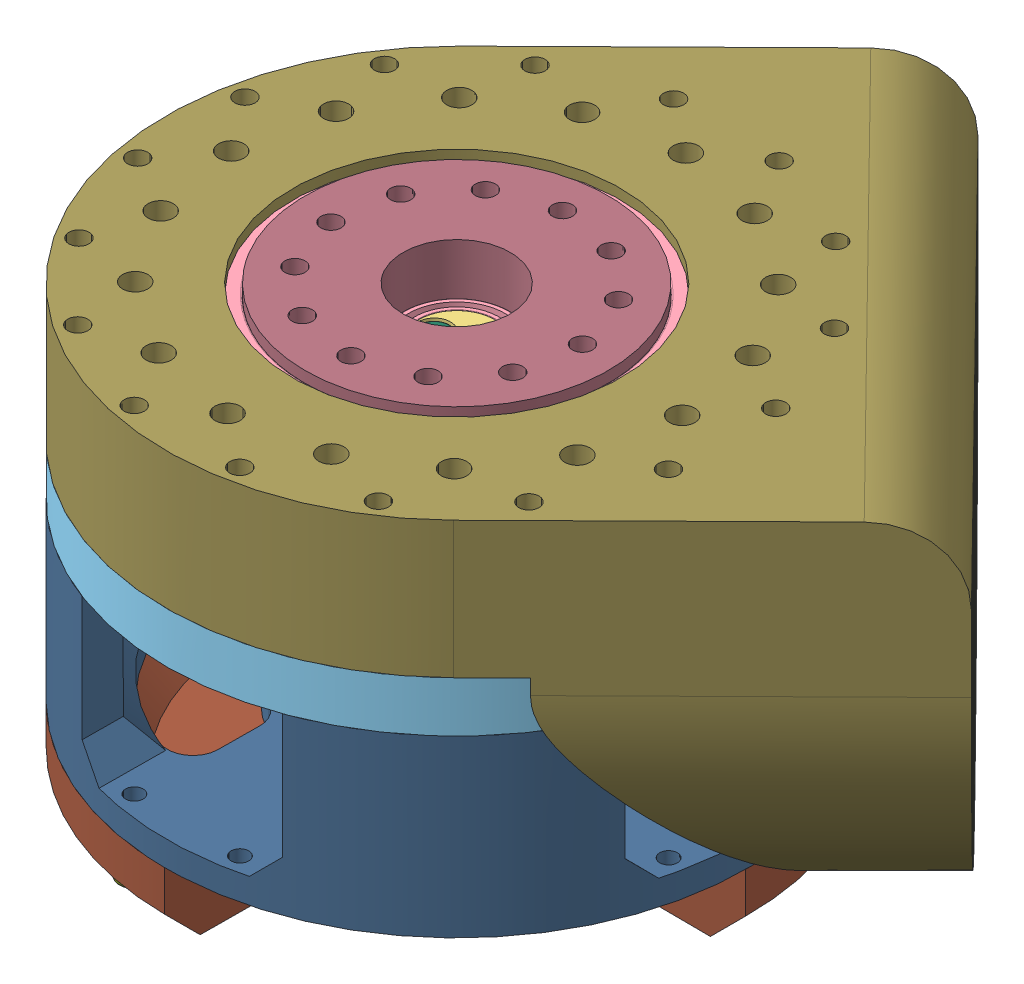
SolidWorks assembly Cycloidal _v3, configuration Default. Lengths in mm.
Overall size (173.36 87.57 173.15).
95 component instances, 17 part files, 90 mates.
Components (placement in the parent):
- motor-X83008S.stp-1: motor-X83008S.stp [Default] at (3.9105 88.7742 94.1058) x (0.928336 0.00037 -0.371741) z (0.000399 -1 0) (suppressed, hidden)
- Base_Plate-1: Base_Plate [Default] at (47.4533 68.6574 89.6282) x (-0.992404 -0.000396 0.123023) z (-0.123023 -0.000049 -0.992404) size (39.8 11 39.8)
- Eccentric_Shaft-1: Eccentric_Shaft [Default] at (60.4961 73.3217 80.3225) x (0.123023 0.000049 0.992404) z (-0.992404 -0.000396 0.123023) size (20 17 17)
  - Eccentric_Shaft_bot-1: Eccentric_Shaft_bot [Default] at (7.6302 12.3409 14.0904) x (1 0 0) z (0 0 -1) size (17 6 17)
  - Eccentric_Shaft_bot-2: Eccentric_Shaft_bot [Default] at (7.6302 12.3409 14.0904) x (-1 0 0) z (0 0 -1) size (17 6 17)
  - Eccentric_Shaft_top-1: Eccentric_Shaft_top [Default] at (7.6302 18.3409 14.0904) x (-1 0 0) z (0 0 -1) size (17 5 17)
- radial ball bearing_68_iso-39: radial ball bearing_68_iso [ISO 15 RBB - 1860 - 32,SI,NC,32_68] at (47.4409 99.6574 89.6282) x (0.000399 -1 0) z (-0.546908 -0.000218 0.837193) size (10 78 78)
- radial ball bearing_68_iso-40: radial ball bearing_68_iso [ISO 15 RBB - 1840 - 32,SI,NC,32_68] at (47.4516 72.9574 89.6282) x (-0.000399 1 0) z (0.001003 0 0.999999) size (7 52 52)
- Base_plate_2-1: Base_plate_2 [Default] at (47.4529 69.6574 89.6282) x (0.712755 0.000284 -0.701413) z (0.701413 0.00028 0.712755) size (115 10 115)
- m13_bearing-31: m13_bearing [Default] at (-10.4263 95.4017 67.196) x (0.227678 0.000091 0.973736) z (0.973736 0.000388 -0.227678) size (13 16 13)
  - m6-1: m6 [Default] at (8.4921 2.5508 14.8914) size (6 16 6)
  - radial ball bearing_68_iso-1: radial ball bearing_68_iso [ISO 15 RBB - 286 - 10,SI,NC,10_68] at (8.4921 16.0508 14.8914) x (0 1 0) z (0 0 1) size (5 13 13)
  - radial ball bearing_68_iso-2: radial ball bearing_68_iso [ISO 15 RBB - 286 - 10,SI,NC,10_68] at (8.4921 11.0508 14.8914) x (0 1 0) z (0 0 1) size (5 13 13)
- m13_bearing-32: m13_bearing [Default] at (-13.9908 98.1837 84.3887) x (0.227678 0.000091 0.973736) z (0.973736 0.000388 -0.227678) size (13 16 13)
  - m6-1: m6 [Default] at (8.4921 2.5508 14.8914) size (6 16 6)
  - radial ball bearing_68_iso-1: radial ball bearing_68_iso [ISO 15 RBB - 286 - 10,SI,NC,10_68] at (8.4921 16.0508 14.8914) x (0 1 0) z (0 0 1) size (5 13 13)
  - radial ball bearing_68_iso-2: radial ball bearing_68_iso [ISO 15 RBB - 286 - 10,SI,NC,10_68] at (8.4921 11.0508 14.8914) x (0 1 0) z (0 0 1) size (5 13 13)
- m13_bearing-34: m13_bearing [Default] at (13.4541 98.1947 126.1847) x (0.227678 0.000091 0.973736) z (0.973736 0.000388 -0.227678) size (13 16 13)
  - m6-1: m6 [Default] at (8.4921 2.5508 14.8914) size (6 16 6)
  - radial ball bearing_68_iso-1: radial ball bearing_68_iso [ISO 15 RBB - 286 - 10,SI,NC,10_68] at (8.4921 16.0508 14.8914) x (0 1 0) z (0 0 1) size (5 13 13)
  - radial ball bearing_68_iso-2: radial ball bearing_68_iso [ISO 15 RBB - 286 - 10,SI,NC,10_68] at (8.4921 11.0508 14.8914) x (0 1 0) z (0 0 1) size (5 13 13)
- m13_bearing-35: m13_bearing [Default] at (-1.0662 98.1889 116.3132) x (0.227678 0.000091 0.973736) z (0.973736 0.000388 -0.227678) size (13 16 13)
  - m6-1: m6 [Default] at (8.4921 2.5508 14.8914) size (6 16 6)
  - radial ball bearing_68_iso-1: radial ball bearing_68_iso [ISO 15 RBB - 286 - 10,SI,NC,10_68] at (8.4921 16.0508 14.8914) x (0 1 0) z (0 0 1) size (5 13 13)
  - radial ball bearing_68_iso-2: radial ball bearing_68_iso [ISO 15 RBB - 286 - 10,SI,NC,10_68] at (8.4921 11.0508 14.8914) x (0 1 0) z (0 0 1) size (5 13 13)
- m13_bearing-36: m13_bearing [Default] at (-10.7036 98.185 101.6364) x (0.227678 0.000091 0.973736) z (0.973736 0.000388 -0.227678) size (13 16 13)
  - m6-1: m6 [Default] at (8.4921 2.5508 14.8914) size (6 16 6)
  - radial ball bearing_68_iso-1: radial ball bearing_68_iso [ISO 15 RBB - 286 - 10,SI,NC,10_68] at (8.4921 16.0508 14.8914) x (0 1 0) z (0 0 1) size (5 13 13)
  - radial ball bearing_68_iso-2: radial ball bearing_68_iso [ISO 15 RBB - 286 - 10,SI,NC,10_68] at (8.4921 11.0508 14.8914) x (0 1 0) z (0 0 1) size (5 13 13)
- m13_bearing-1: m13_bearing [Default] at (-0.4494 98.1891 62.778) x (0.736525 0.000294 0.676411) z (0.676411 0.00027 -0.736525) size (13 16 13)
  - m6-1: m6 [Default] at (8.4921 2.5508 14.8914) size (6 16 6)
  - radial ball bearing_68_iso-1: radial ball bearing_68_iso [ISO 15 RBB - 286 - 10,SI,NC,10_68] at (8.4921 16.0508 14.8914) x (0 1 0) z (0 0 1) size (5 13 13)
  - radial ball bearing_68_iso-2: radial ball bearing_68_iso [ISO 15 RBB - 286 - 10,SI,NC,10_68] at (8.4921 11.0508 14.8914) x (0 1 0) z (0 0 1) size (5 13 13)
- m13_bearing-2: m13_bearing [Default] at (48.5236 98.2087 124.7001) x (0.120271 0.000048 0.992741) z (0.992741 0.000396 -0.120271) size (13 16 13)
  - m6-1: m6 [Default] at (8.4921 2.5508 14.8914) size (6 16 6)
  - radial ball bearing_68_iso-1: radial ball bearing_68_iso [ISO 15 RBB - 286 - 10,SI,NC,10_68] at (8.4921 16.0508 14.8914) x (0 1 0) z (0 0 1) size (5 13 13)
  - radial ball bearing_68_iso-2: radial ball bearing_68_iso [ISO 15 RBB - 286 - 10,SI,NC,10_68] at (8.4921 11.0508 14.8914) x (0 1 0) z (0 0 1) size (5 13 13)
- m13_bearing-3: m13_bearing [Default] at (32.5019 98.2023 52.3604) x (0.833889 0.000333 0.551933) z (0.551932 0.00022 -0.833889) size (13 16 13)
  - m6-1: m6 [Default] at (8.4921 2.5508 14.8914) size (6 16 6)
  - radial ball bearing_68_iso-1: radial ball bearing_68_iso [ISO 15 RBB - 286 - 10,SI,NC,10_68] at (8.4921 16.0508 14.8914) x (0 1 0) z (0 0 1) size (5 13 13)
  - radial ball bearing_68_iso-2: radial ball bearing_68_iso [ISO 15 RBB - 286 - 10,SI,NC,10_68] at (8.4921 11.0508 14.8914) x (0 1 0) z (0 0 1) size (5 13 13)
- m13_bearing-4: m13_bearing [Default] at (77.3632 98.2202 81.8307) x (0.022268 0.000009 0.999752) z (0.999752 0.000399 -0.022268) size (13 16 13)
  - m6-1: m6 [Default] at (8.4921 2.5508 14.8914) size (6 16 6)
  - radial ball bearing_68_iso-1: radial ball bearing_68_iso [ISO 15 RBB - 286 - 10,SI,NC,10_68] at (8.4921 16.0508 14.8914) x (0 1 0) z (0 0 1) size (5 13 13)
  - radial ball bearing_68_iso-2: radial ball bearing_68_iso [ISO 15 RBB - 286 - 10,SI,NC,10_68] at (8.4921 11.0508 14.8914) x (0 1 0) z (0 0 1) size (5 13 13)
- m13_bearing-5: m13_bearing [Default] at (73.5091 98.2186 99.5852) x (0.059133 0.000024 0.99825) z (0.99825 0.000398 -0.059133) size (13 16 13)
  - m6-1: m6 [Default] at (8.4921 2.5508 14.8914) size (6 16 6)
  - radial ball bearing_68_iso-1: radial ball bearing_68_iso [ISO 15 RBB - 286 - 10,SI,NC,10_68] at (8.4921 16.0508 14.8914) x (0 1 0) z (0 0 1) size (5 13 13)
  - radial ball bearing_68_iso-2: radial ball bearing_68_iso [ISO 15 RBB - 286 - 10,SI,NC,10_68] at (8.4921 11.0508 14.8914) x (0 1 0) z (0 0 1) size (5 13 13)
- m13_bearing-6: m13_bearing [Default] at (13.4333 98.1947 47.0643) x (0.451561 0.00018 0.89224) z (0.89224 0.000356 -0.451561) size (13 16 13)
  - m6-1: m6 [Default] at (8.4921 2.5508 14.8914) size (6 16 6)
  - radial ball bearing_68_iso-1: radial ball bearing_68_iso [ISO 15 RBB - 286 - 10,SI,NC,10_68] at (8.4921 16.0508 14.8914) x (0 1 0) z (0 0 1) size (5 13 13)
  - radial ball bearing_68_iso-2: radial ball bearing_68_iso [ISO 15 RBB - 286 - 10,SI,NC,10_68] at (8.4921 11.0508 14.8914) x (0 1 0) z (0 0 1) size (5 13 13)
- m13_bearing-7: m13_bearing [Default] at (57.1526 98.2121 32.9496) x (-0.545813 -0.000218 0.837907) z (0.837907 0.000334 0.545813) size (13 16 13)
  - m6-1: m6 [Default] at (8.4921 2.5508 14.8914) size (6 16 6)
  - radial ball bearing_68_iso-1: radial ball bearing_68_iso [ISO 15 RBB - 286 - 10,SI,NC,10_68] at (8.4921 16.0508 14.8914) x (0 1 0) z (0 0 1) size (5 13 13)
  - radial ball bearing_68_iso-2: radial ball bearing_68_iso [ISO 15 RBB - 286 - 10,SI,NC,10_68] at (8.4921 11.0508 14.8914) x (0 1 0) z (0 0 1) size (5 13 13)
- m13_bearing-8: m13_bearing [Default] at (73.1034 98.2185 66.7178) x (0.158553 0.000063 0.98735) z (0.98735 0.000394 -0.158553) size (13 16 13)
  - m6-1: m6 [Default] at (8.4921 2.5508 14.8914) size (6 16 6)
  - radial ball bearing_68_iso-1: radial ball bearing_68_iso [ISO 15 RBB - 286 - 10,SI,NC,10_68] at (8.4921 16.0508 14.8914) x (0 1 0) z (0 0 1) size (5 13 13)
  - radial ball bearing_68_iso-2: radial ball bearing_68_iso [ISO 15 RBB - 286 - 10,SI,NC,10_68] at (8.4921 11.0508 14.8914) x (0 1 0) z (0 0 1) size (5 13 13)
- m13_bearing-9: m13_bearing [Default] at (74.5316 98.219 41.6624) x (-0.687134 -0.000274 0.72653) z (0.72653 0.00029 0.687134) size (13 16 13)
  - m6-1: m6 [Default] at (8.4921 2.5508 14.8914) size (6 16 6)
  - radial ball bearing_68_iso-1: radial ball bearing_68_iso [ISO 15 RBB - 286 - 10,SI,NC,10_68] at (8.4921 16.0508 14.8914) x (0 1 0) z (0 0 1) size (5 13 13)
  - radial ball bearing_68_iso-2: radial ball bearing_68_iso [ISO 15 RBB - 286 - 10,SI,NC,10_68] at (8.4921 11.0508 14.8914) x (0 1 0) z (0 0 1) size (5 13 13)
- m13_bearing-11: m13_bearing [Default] at (30.0113 98.2013 136.2104) x (0.57351 0.000229 0.819198) z (0.819198 0.000327 -0.57351) size (13 16 13)
  - m6-1: m6 [Default] at (8.4921 2.5508 14.8914) size (6 16 6)
  - radial ball bearing_68_iso-1: radial ball bearing_68_iso [ISO 15 RBB - 286 - 10,SI,NC,10_68] at (8.4921 16.0508 14.8914) x (0 1 0) z (0 0 1) size (5 13 13)
  - radial ball bearing_68_iso-2: radial ball bearing_68_iso [ISO 15 RBB - 286 - 10,SI,NC,10_68] at (8.4921 11.0508 14.8914) x (0 1 0) z (0 0 1) size (5 13 13)
- m13_bearing-12: m13_bearing [Default] at (62.5932 98.2143 116.7506) x (0.22335 0.000089 0.974738) z (0.974738 0.000389 -0.22335) size (13 16 13)
  - m6-1: m6 [Default] at (8.4921 2.5508 14.8914) size (6 16 6)
  - radial ball bearing_68_iso-1: radial ball bearing_68_iso [ISO 15 RBB - 286 - 10,SI,NC,10_68] at (8.4921 16.0508 14.8914) x (0 1 0) z (0 0 1) size (5 13 13)
  - radial ball bearing_68_iso-2: radial ball bearing_68_iso [ISO 15 RBB - 286 - 10,SI,NC,10_68] at (8.4921 11.0508 14.8914) x (0 1 0) z (0 0 1) size (5 13 13)
- M3x4x4.2_brass_insert-22: M3x4x4.2_brass_insert [Default] at (43.4837 68.6558 90.1203) x (0.984609 0.000393 -0.174769) z (0.174769 0.00007 0.984609) size (4 4 4)
- M3x4x4.2_brass_insert-23: M3x4x4.2_brass_insert [Default] at (51.4229 68.659 89.1361) x (0.984609 0.000393 -0.174769) z (0.174769 0.00007 0.984609) size (4 4 4)
- radial ball bearing_68_iso-44: radial ball bearing_68_iso [ISO 15 RBB - 1715 - 26,SI,NC,26_68] at (47.2636 81.6573 88.1396) x (0.000399 -1 0) z (0.171535 0.000068 0.985178) size (4 21 21)
- radial ball bearing_68_iso-45: radial ball bearing_68_iso [ISO 15 RBB - 1715 - 26,SI,NC,26_68] at (47.4429 94.6574 89.6282) x (0.000399 -1 0) z (0.819169 0.000327 0.573552) size (4 21 21)
- radial ball bearing_68_iso-46: radial ball bearing_68_iso [ISO 15 RBB - 1715 - 26,SI,NC,26_68] at (47.6295 89.6575 91.1168) x (-0.000399 1 0) z (0 0 1) size (4 21 21)
- foc-motor-controller.step-1: foc-motor-controller.step [Default] at (47.4677 32.6574 89.6282) x (0.701413 0.00028 0.712755) z (0.000399 -1 0) (suppressed, hidden)
- hex nut style 1 gradeab_iso-1: hex nut style 1 gradeab_iso [ISO - 4032 - M3 - W - N] at (47.7115 32.6575 59.2236) x (1 0.000399 0) z (0.000399 -1 0) size (5.5 6.35 2.4)
- Cycloidal_Discs_8308-1: Cycloidal_Discs_8308 [Default] at (-11.9184 124.164 51.5043) x (0.028527 0.000011 0.999593) z (0.999593 0.000399 -0.028527) size (79.25 5 79.73)
  - Cycloidal_Discs-1: Cycloidal_Discs [Default] at (38.3081 39.5303 58.0959) size (79.25 5 79.73)
- Cycloidal_Discs_8308-2: Cycloidal_Discs_8308 [Default] at (62.1667 47.133 159.1742) x (-0.931329 -0.000371 -0.364178) z (0.364178 0.000145 -0.931329) size (79.25 5 79.73)
  - Cycloidal_Discs-1: Cycloidal_Discs [Default] at (38.3081 39.5303 58.0959) size (79.25 5 79.73)
- Motor_Cover_v2-2: Motor_Cover_v2 [Default] at (47.4667 35.0574 89.6282) x (0.999968 0.000399 0.00802) z (-0.00802 -0.000003 0.999968) size (115 34.6 115)
- driver_cover-1: driver_cover [Default] at (47.4667 35.0574 89.6282) x (0.702656 0.00028 0.711529) z (0.711529 0.000284 -0.702656) size (81.32 15 115)
- Cover_new-1: Cover_new [Default] at (47.4437 92.6574 89.6282) x (0.701413 0.00028 0.712755) z (-0.712755 -0.000284 0.701413) size (115 87.5 130)
- Output_Shaft-2: Output_Shaft [Default] at (47.4437 92.6574 89.6282) x (0.572675 0.000228 0.819783) z (-0.819783 -0.000327 0.572675) size (70 14 70)
- radial ball bearing_68_iso-47: radial ball bearing_68_iso [ISO 15 RBB - 289 - 14,SI,NC,14_68] at (61.9924 89.1632 109.081) x (0.000399 -1 0) z (-0.055662 -0.000022 0.99845) size (5 17 17)
- radial ball bearing_68_iso-48: radial ball bearing_68_iso [ISO 15 RBB - 289 - 14,SI,NC,14_68] at (59.3269 82.1622 107.722) x (0.000399 -1 0) z (-0.055662 -0.000022 0.99845) size (5 17 17)
- m4x14-1: m4x14 [Default] at (47.0925 68.4573 134.6267) x (0.999623 0.000399 0.027466) z (-0.027466 -0.000011 0.999623) size (8 15.2 8)
- M3x20-1: M3x20 [Default] at (43.4726 96.3558 90.1203) x (-0.837193 -0.000334 -0.546908) z (-0.546908 -0.000218 0.837193) size (6 21.2 6)
- M3x10-1: M3x10 [Default] at (36.5111 25.853 142.5044) x (0.424034 0.000169 -0.905646) z (0.905646 0.000361 0.424034) size (6 11.2 6)
- m3x60-1: m3x60 [Default] at (17.1068 35.0453 134.2855) x (-0.837193 -0.000334 -0.546908) z (-0.546908 -0.000218 0.837193) size (5.3 63 5.3)
- m6-1: m6 [Default] at (60.6129 98.6627 108.4832) x (-0.153131 -0.000061 0.988206) z (0.988206 0.000394 0.153131) size (6 16 6)
Mates (geometry in assembly coordinates):
- Coincident1: coincident anti-aligned: plane of motor-X83008S.stp-1/outrunner.stp-1 through (51.6976 68.6591 123.8661) normal (-0.000399 1 0); plane of Base_Plate-1 through (47.4533 68.6574 89.6282) normal (0.000399 -1 0)
- Concentric1: concentric anti-aligned: line of motor-X83008S.stp-1/outrunner.stp-1 through (49.3624 63.1582 105.0104) axis (-0.000399 1 0); cylinder of Base_Plate-1 through (49.3558 79.6582 105.0104) axis (0.000399 -1 0) radius 2
- Concentric2: concentric anti-aligned: cylinder of motor-X83008S.stp-1/shaft.stp-1 through (47.4533 68.6574 89.6282) axis (-0.000399 1 0) radius 1.5; line of Base_Plate-1 through (47.4489 79.6574 89.6282) axis (0.000399 -1 0)
- Concentric78: concentric anti-aligned: cylinder of Base_Plate-1 through (47.4489 79.6574 89.6282) axis (0.000399 -1 0) radius 19.9; cylinder of radial ball bearing_68_iso-40 through (47.4598 52.3199 89.6282) axis (-0.000399 1 0) radius 20
- Concentric1437: concentric anti-aligned: cylinder of Base_Plate-1 through (43.4793 79.6558 90.1203) axis (0.000399 -1 0) radius 2; cylinder of M3x4x4.2_brass_insert-22 through (43.4817 73.5579 90.1203) axis (-0.000399 1 0) radius 1.5
- Coincident1479: coincident aligned: plane of Base_Plate-1 through (47.4533 68.6574 89.6282) normal (0.000399 -1 0); plane of M3x4x4.2_brass_insert-22 through (44.9606 68.6564 89.8581) normal (0.000399 -1 0)
- Concentric1438: concentric anti-aligned: cylinder of Base_Plate-1 through (51.4185 79.659 89.1361) axis (0.000399 -1 0) radius 2; cylinder of M3x4x4.2_brass_insert-23 through (51.421 73.561 89.1361) axis (-0.000399 1 0) radius 1.5
- Coincident1480: coincident aligned: plane of Base_Plate-1 through (47.4533 68.6574 89.6282) normal (0.000399 -1 0); plane of M3x4x4.2_brass_insert-23 through (52.8998 68.6596 88.8739) normal (0.000399 -1 0)
- Concentric1445038: concentric anti-aligned: cylinder of Base_Plate-1 through (47.4489 79.6574 89.6282) axis (0.000399 -1 0) radius 19.9; cylinder of radial ball bearing_68_iso-40 through (47.4598 52.3199 89.6282) axis (-0.000399 1 0) radius 20
- Coincident1486651: coincident aligned: plane of Base_Plate-1 through (47.4489 79.6574 89.6282) normal (-0.000399 1 0); plane of Base_plate_2-1 through (47.4489 79.6574 89.6282) normal (-0.000399 1 0)
- Concentric1445041: concentric anti-aligned: cylinder of radial ball bearing_68_iso-40 through (47.4598 52.3199 89.6282) axis (-0.000399 1 0) radius 26; cylinder of Base_plate_2-1 through (47.4489 79.6574 89.6282) axis (0.000399 -1 0) radius 26.1
- Concentric1445057: concentric aligned: cylinder of Base_plate_2-1 through (6.0138 79.6409 72.0746) axis (0.000399 -1 0) radius 2.1; cylinder of m13_bearing-31/radial ball bearing_68_iso-2 through (6.0037 104.995 72.0746) axis (0.000399 -1 0) radius 6.5
- Coincident1486692: coincident anti-aligned: plane of foc-motor-controller.step-1/foc-motor-controller_PCB.step-1 through (47.4677 32.6574 89.6282) normal (-0.000399 1 0); plane of hex nut style 1 gradeab_iso-1 through (47.7115 32.6575 62.399) normal (0.000399 -1 0)
- Concentric14450545: concentric anti-aligned: cylinder of radial ball bearing_68_iso-46 through (47.6377 69.02 91.1168) axis (-0.000399 1 0) radius 10.5; cylinder of Cycloidal_Discs_8308-2/Cycloidal_Discs-1 through (47.6287 91.6575 91.1168) axis (0.000399 -1 0) radius 10.6
- Coincident1486693: coincident aligned: plane of radial ball bearing_68_iso-46 through (37.3287 91.6534 91.1168) normal (-0.000399 1 0); plane of Cycloidal_Discs_8308-2/Cycloidal_Discs-1 through (33.5025 91.6519 126.7829) normal (-0.000399 1 0)
- Concentric14450546: concentric anti-aligned: cylinder of radial ball bearing_68_iso-44 through (47.2554 102.2948 88.1396) axis (0.000399 -1 0) radius 10.5; cylinder of Cycloidal_Discs_8308-1/Cycloidal_Discs-1 through (47.2644 79.6573 88.1396) axis (-0.000399 1 0) radius 10.6
- Concentric14450559: concentric anti-aligned: cylinder of foc-motor-controller.step-1/foc-motor-controller_PCB.step-1 through (47.2238 32.7033 120.0328) axis (-0.000399 1 0) radius 1.6; cylinder of Motor_Cover_v2-2 through (47.2029 85.0573 120.0328) axis (0.000399 -1 0) radius 1.5
- Concentric14450560: concentric anti-aligned: circle of foc-motor-controller.step-1/foc-motor-controller_PCB.step-1; cylinder of Motor_Cover_v2-2 through (47.6906 85.0575 59.2236) axis (0.000399 -1 0) radius 1.5
- Coincident1486699: coincident anti-aligned: line of foc-motor-controller.step-1/foc-motor-controller_PCB.step-1 through (47.7121 31.1475 59.2236) axis (-0.000399 1 0); line of hex nut style 1 gradeab_iso-1 through (47.7106 34.8571 59.2236) axis (0.000399 -1 0)
- Coincident1486700: coincident aligned: circle of hex nut style 1 gradeab_iso-1; plane of Motor_Cover_v2-2 through (47.4667 35.0574 89.6282) normal (0.000399 -1 0)
- Concentric14450561: concentric anti-aligned: cylinder of Motor_Cover_v2-2 through (47.4529 69.6574 89.6282) axis (0.000399 -1 0) radius 57.5; cylinder of driver_cover-1 through (47.4727 20.0574 89.6282) axis (-0.000399 1 0) radius 57.5
- Coincident1486701: coincident anti-aligned: plane of Motor_Cover_v2-2 through (47.4667 35.0574 89.6282) normal (0.000399 -1 0); plane of driver_cover-1 through (47.4667 35.0574 89.6282) normal (-0.000399 1 0)
- Concentric14450563: concentric anti-aligned: cylinder of Eccentric_Shaft-1/Eccentric_Shaft_bot-1 through (47.2644 79.6573 88.1396) axis (-0.000399 1 0) radius 7.5; cylinder of radial ball bearing_68_iso-44 through (47.2554 102.2948 88.1396) axis (0.000399 -1 0) radius 7.5
- Concentric14450564: concentric anti-aligned: cylinder of Eccentric_Shaft-1/Eccentric_Shaft_bot-2 through (47.6287 91.6575 91.1168) axis (0.000399 -1 0) radius 7.5; cylinder of radial ball bearing_68_iso-46 through (47.6377 69.02 91.1168) axis (-0.000399 1 0) radius 7.5
- Coincident1486703: coincident anti-aligned: plane of Eccentric_Shaft-1/Eccentric_Shaft_top-1 through (47.4441 91.6574 89.6282) normal (0.000399 -1 0); plane of Cycloidal_Discs_8308-2/Cycloidal_Discs-1 through (33.5025 91.6519 126.7829) normal (-0.000399 1 0)
- Coincident1486704: coincident aligned: plane of Eccentric_Shaft-1/Eccentric_Shaft_bot-1 through (47.2644 79.6573 88.1396) normal (0.000399 -1 0); circle of radial ball bearing_68_iso-44
- Concentric14450565: concentric aligned: cylinder of Eccentric_Shaft-1/Eccentric_Shaft_top-1 through (47.4421 96.6574 89.6282) axis (0.000399 -1 0) radius 7.5; cylinder of radial ball bearing_68_iso-45 through (47.4347 115.2949 89.6282) axis (0.000399 -1 0) radius 7.5
- Coincident1486705: coincident anti-aligned: plane of Eccentric_Shaft-1/Eccentric_Shaft_top-1 through (47.4421 96.6574 89.6282) normal (-0.000399 1 0); circle of radial ball bearing_68_iso-45
- Coincident1486706: coincident aligned: plane of Eccentric_Shaft-1/Eccentric_Shaft_bot-1 through (47.2644 79.6573 88.1396) normal (0.000399 -1 0); plane of Cycloidal_Discs_8308-1/Cycloidal_Discs-1 through (8.9234 79.642 89.4011) normal (0.000399 -1 0)
- Concentric14450566: concentric aligned: cylinder of Base_plate_2-1 through (47.4489 79.6574 89.6282) axis (0.000399 -1 0) radius 57.5; cylinder of radial ball bearing_68_iso-45 through (47.4347 115.2949 89.6282) axis (0.000399 -1 0) radius 10.5
- Coincident1486707: coincident anti-aligned: line of Base_Plate-1 through (43.4793 79.6558 90.1203) axis (0.000399 -1 0); line of Eccentric_Shaft-1/Eccentric_Shaft_top-1 through (43.4731 95.1558 90.1203) axis (-0.000399 1 0)
- Coincident1486708: coincident anti-aligned: plane of Base_Plate-1 through (47.4489 79.6574 89.6282) normal (-0.000399 1 0); plane of Eccentric_Shaft-1/Eccentric_Shaft_bot-1 through (47.2644 79.6573 88.1396) normal (0.000399 -1 0)
- Concentric14450567: concentric aligned: line of Base_plate_2-1 through (92.4475 79.6754 89.9891) axis (0.000399 -1 0); cylinder of m13_bearing-4/radial ball bearing_68_iso-2 through (92.4363 107.8129 89.9891) axis (0.000399 -1 0) radius 6.5
- Concentric14450568: concentric aligned: circle of Base_plate_2-1; line of m13_bearing-5/m6-1 through (88.884 79.7739 107.1818) axis (-0.000399 1 0)
- Concentric14450569: concentric aligned: circle of Base_plate_2-1; cylinder of m13_bearing-12/m6-1 through (79.0085 89.67 121.7021) axis (-0.000399 1 0) radius 2
- Concentric14450570: concentric anti-aligned: cylinder of Base_plate_2-1 through (64.3357 79.6641 131.3395) axis (0.000399 -1 0) radius 2.1; cylinder of m13_bearing-2/m6-1 through (64.3317 89.6641 131.3395) axis (-0.000399 1 0) radius 2
- Concentric14450571: concentric anti-aligned: cylinder of Base_plate_2-1 through (47.088 79.6573 134.6267) axis (0.000399 -1 0) radius 2.1; cylinder of m13_bearing-11/m6-1 through (47.0841 89.6573 134.6267) axis (-0.000399 1 0) radius 2
- Concentric14450572: concentric anti-aligned: cylinder of Base_plate_2-1 through (29.8953 79.6504 131.0633) axis (0.000399 -1 0) radius 2.1; cylinder of m13_bearing-34/m6-1 through (29.8913 89.6504 131.0633) axis (-0.000399 1 0) radius 2
- Concentric14450573: concentric anti-aligned: cylinder of Base_plate_2-1 through (15.375 79.6446 121.1918) axis (0.000399 -1 0) radius 2.1; cylinder of m13_bearing-35/m6-1 through (15.371 89.6446 121.1918) axis (-0.000399 1 0) radius 2
- Concentric14450574: concentric anti-aligned: cylinder of Base_plate_2-1 through (5.7376 79.6408 106.515) axis (0.000399 -1 0) radius 2.1; cylinder of m13_bearing-36/m6-1 through (5.7336 89.6408 106.515) axis (-0.000399 1 0) radius 2
- Concentric14450575: concentric anti-aligned: cylinder of Base_plate_2-1 through (2.4504 79.6395 89.2673) axis (0.000399 -1 0) radius 2.1; cylinder of m13_bearing-32/m6-1 through (2.4464 89.6395 89.2673) axis (-0.000399 1 0) radius 2
- Concentric14450576: concentric anti-aligned: cylinder of Base_plate_2-1 through (6.0138 79.6409 72.0746) axis (0.000399 -1 0) radius 2.1; cylinder of m13_bearing-31/m6-1 through (6.0109 86.8575 72.0746) axis (-0.000399 1 0) radius 2
- Concentric14450577: concentric anti-aligned: cylinder of Base_plate_2-1 through (15.8853 79.6448 57.5542) axis (0.000399 -1 0) radius 2.1; cylinder of m13_bearing-1/m6-1 through (15.8813 89.6448 57.5542) axis (-0.000399 1 0) radius 2
- Concentric14450578: concentric anti-aligned: cylinder of Base_plate_2-1 through (30.5621 79.6507 47.9168) axis (0.000399 -1 0) radius 2.1; cylinder of m13_bearing-6/m6-1 through (30.5581 89.6507 47.9168) axis (-0.000399 1 0) radius 2
- Concentric14450579: concentric anti-aligned: cylinder of Base_plate_2-1 through (47.8098 79.6576 44.6296) axis (0.000399 -1 0) radius 2.1; line of m13_bearing-3/m6-1 through (47.8058 89.6576 44.6296) axis (-0.000399 1 0)
- Concentric14450580: concentric anti-aligned: cylinder of Base_plate_2-1 through (65.0025 79.6644 48.193) axis (0.000399 -1 0) radius 2.1; cylinder of m13_bearing-7/m6-1 through (64.9985 89.6644 48.193) axis (-0.000399 1 0) radius 2
- Concentric14450581: concentric anti-aligned: cylinder of Base_plate_2-1 through (79.5229 79.6702 58.0646) axis (0.000399 -1 0) radius 2.1; cylinder of m13_bearing-9/m6-1 through (79.5189 89.6702 58.0646) axis (-0.000399 1 0) radius 2
- Concentric14450582: concentric anti-aligned: cylinder of Base_plate_2-1 through (89.1603 79.6741 72.7414) axis (0.000399 -1 0) radius 2.1; cylinder of m13_bearing-8/m6-1 through (89.1563 89.674 72.7414) axis (-0.000399 1 0) radius 2
- Coincident1486709: coincident anti-aligned: plane of Base_plate_2-1 through (47.4489 79.6574 89.6282) normal (-0.000399 1 0); circle of m13_bearing-32/m6-1
- Coincident1486710: coincident anti-aligned: plane of Base_plate_2-1 through (47.4489 79.6574 89.6282) normal (-0.000399 1 0); circle of m13_bearing-3/radial ball bearing_68_iso-1
- Coincident1486711: coincident anti-aligned: plane of Base_plate_2-1 through (47.4489 79.6574 89.6282) normal (-0.000399 1 0); circle of m13_bearing-5/radial ball bearing_68_iso-1
- Coincident1486712: coincident anti-aligned: plane of Base_plate_2-1 through (47.4489 79.6574 89.6282) normal (-0.000399 1 0); circle of m13_bearing-11/radial ball bearing_68_iso-1
- Coincident1486713: coincident anti-aligned: plane of Base_plate_2-1 through (47.4489 79.6574 89.6282) normal (-0.000399 1 0); circle of m13_bearing-34/m6-1
- Coincident1486714: coincident anti-aligned: plane of Base_plate_2-1 through (47.4489 79.6574 89.6282) normal (-0.000399 1 0); circle of m13_bearing-35/m6-1
- Coincident1486715: coincident anti-aligned: plane of Base_plate_2-1 through (47.4489 79.6574 89.6282) normal (-0.000399 1 0); circle of m13_bearing-36/m6-1
- Coincident1486716: coincident anti-aligned: plane of Base_plate_2-1 through (47.4489 79.6574 89.6282) normal (-0.000399 1 0); circle of m13_bearing-2/m6-1
- Coincident1486717: coincident anti-aligned: plane of Base_plate_2-1 through (47.4489 79.6574 89.6282) normal (-0.000399 1 0); circle of m13_bearing-12/m6-1
- Coincident1486718: coincident anti-aligned: plane of Base_plate_2-1 through (47.4489 79.6574 89.6282) normal (-0.000399 1 0); circle of m13_bearing-6/m6-1
- Coincident1486719: coincident anti-aligned: plane of Base_plate_2-1 through (47.4489 79.6574 89.6282) normal (-0.000399 1 0); circle of m13_bearing-4/m6-1
- Coincident1486720: coincident anti-aligned: plane of Base_plate_2-1 through (47.4489 79.6574 89.6282) normal (-0.000399 1 0); circle of m13_bearing-8/m6-1
- Coincident1486721: coincident anti-aligned: plane of Base_plate_2-1 through (47.4489 79.6574 89.6282) normal (-0.000399 1 0); circle of m13_bearing-9/m6-1
- Coincident1486722: coincident anti-aligned: plane of Base_plate_2-1 through (47.4489 79.6574 89.6282) normal (-0.000399 1 0); plane of m13_bearing-7/m6-1 through (65.0025 79.6644 48.193) normal (0.000399 -1 0)
- Coincident1486723: coincident anti-aligned: plane of Base_plate_2-1 through (47.4489 79.6574 89.6282) normal (-0.000399 1 0); circle of m13_bearing-1/m6-1
- Concentric14450583: concentric aligned: cylinder of Base_plate_2-1 through (47.4489 79.6574 89.6282) axis (0.000399 -1 0) radius 57.5; cylinder of Cover_new-1 through (47.4382 106.6574 89.6282) axis (0.000399 -1 0) radius 57.5
- Concentric14450586: concentric aligned: cylinder of Base_plate_2-1 through (47.4489 79.6574 89.6282) axis (0.000399 -1 0) radius 57.5; cylinder of Motor_Cover_v2-2 through (47.4529 69.6574 89.6282) axis (0.000399 -1 0) radius 57.5
- Concentric14450587: concentric anti-aligned: cylinder of Motor_Cover_v2-2 through (92.5853 85.0754 59.9884) axis (0.000399 -1 0) radius 1.75; circle of Cover_new-1
- Concentric14450588: concentric aligned: cylinder of Motor_Cover_v2-2 through (77.8067 85.0695 44.9709) axis (0.000399 -1 0) radius 1.75; cylinder of driver_cover-1 through (77.8298 27.0695 44.9709) axis (0.000399 -1 0) radius 3.25
- Concentric14450589: concentric aligned: cylinder of radial ball bearing_68_iso-39 through (47.4327 120.2949 89.6282) axis (0.000399 -1 0) radius 30; line of Cover_new-1 through (47.439 104.6574 89.6282) axis (0.000399 -1 0)
- Coincident1486724: coincident anti-aligned: plane of radial ball bearing_68_iso-39 through (74.8152 104.6683 107.5121) normal (-0.000399 1 0); plane of Cover_new-1 through (47.439 104.6574 89.6282) normal (0.000399 -1 0)
- Concentric14450590: concentric aligned: cylinder of radial ball bearing_68_iso-39 through (47.4327 120.2949 89.6282) axis (0.000399 -1 0) radius 30; cylinder of Output_Shaft-2 through (47.4382 106.6574 89.6282) axis (0.000399 -1 0) radius 30
- Coincident1486725: coincident anti-aligned: plane of radial ball bearing_68_iso-39 through (72.8099 94.6675 106.1995) normal (0.000399 -1 0); plane of Output_Shaft-2 through (47.4429 94.6574 89.6282) normal (-0.000399 1 0)
- Concentric14450591: concentric aligned: cylinder of Base_plate_2-1 through (92.5874 79.6754 59.9884) axis (0.000399 -1 0) radius 1.75; cylinder of Motor_Cover_v2-2 through (92.5853 85.0754 59.9884) axis (0.000399 -1 0) radius 1.75
- Concentric14450592: concentric aligned: cylinder of Cycloidal_Discs_8308-2/Cycloidal_Discs-1 through (61.9914 91.6632 109.081) axis (0.000399 -1 0) radius 8.6; cylinder of radial ball bearing_68_iso-47 through (61.9842 109.8007 109.081) axis (0.000399 -1 0) radius 4.5
- Coincident1486726: coincident anti-aligned: plane of Cycloidal_Discs_8308-2/Cycloidal_Discs-1 through (33.5025 91.6519 126.7829) normal (-0.000399 1 0); circle of radial ball bearing_68_iso-47
- Concentric14450593: concentric anti-aligned: cylinder of Cycloidal_Discs_8308-1/Cycloidal_Discs-1 through (59.3279 79.6622 107.722) axis (-0.000399 1 0) radius 8.6; cylinder of radial ball bearing_68_iso-48 through (59.3187 102.7996 107.722) axis (0.000399 -1 0) radius 4.5
- Coincident1486727: coincident aligned: plane of Cycloidal_Discs_8308-1/Cycloidal_Discs-1 through (8.9214 84.642 89.4011) normal (-0.000399 1 0); plane of radial ball bearing_68_iso-48 through (66.6146 84.6651 108.1283) normal (-0.000399 1 0)
- Coincident1486728: coincident anti-aligned: plane of Base_plate_2-1 through (47.4489 79.6574 89.6282) normal (-0.000399 1 0); plane of Cover_new-1 through (47.4489 79.6574 89.6282) normal (0.000399 -1 0)
- Coincident1486730: coincident anti-aligned: plane of motor-X83008S.stp-1/base.stp-1 through (47.4647 40.0574 89.6282) normal (0.000399 -1 0); plane of Motor_Cover_v2-2 through (47.4647 40.0574 89.6282) normal (-0.000399 1 0)
- Concentric14450594: concentric aligned: cylinder of Base_plate_2-1 through (47.088 79.6573 134.6267) axis (0.000399 -1 0) radius 2.1; cylinder of m4x14-1 through (47.0864 83.6573 134.6267) axis (0.000399 -1 0) radius 2
- Coincident1486731: coincident anti-aligned: plane of Base_plate_2-1 through (47.4529 69.6574 89.6282) normal (0.000399 -1 0); plane of m4x14-1 through (47.092 69.6573 134.6267) normal (-0.000399 1 0)
- Coincident1486734: coincident anti-aligned: plane of Eccentric_Shaft-1/Eccentric_Shaft_top-1 through (43.4731 95.1558 90.1203) normal (-0.000399 1 0); plane of M3x20-1 through (40.9615 95.1548 88.4795) normal (0.000399 -1 0)
- Concentric14450595: concentric anti-aligned: cylinder of Eccentric_Shaft-1/Eccentric_Shaft_top-1 through (43.4731 95.1558 90.1203) axis (-0.000399 1 0) radius 3.25; cylinder of M3x20-1 through (43.5018 23.2416 90.1203) axis (0.000399 -1 0) radius 1.5
- Concentric14450596: concentric anti-aligned: cylinder of driver_cover-1 through (36.5074 35.053 142.5044) axis (0.000399 -1 0) radius 1.75; cylinder of M3x10-1 through (36.4819 98.9673 142.5044) axis (-0.000399 1 0) radius 1.5
- Coincident1486735: coincident anti-aligned: plane of driver_cover-1 through (36.5106 27.053 142.5044) normal (0.000399 -1 0); plane of M3x10-1 through (37.7827 27.0536 139.7875) normal (-0.000399 1 0)
- Coincident1486736: coincident anti-aligned: plane of Motor_Cover_v2-2 through (47.4667 35.0574 89.6282) normal (0.000399 -1 0); plane of m3x60-1 through (17.1068 35.0453 134.2855) normal (-0.000399 1 0)
- Concentric14450597: concentric anti-aligned: cylinder of Motor_Cover_v2-2 through (17.0869 85.0453 134.2855) axis (0.000399 -1 0) radius 1.75; cylinder of m3x60-1 through (17.108 32.0453 134.2855) axis (-0.000399 1 0) radius 2.65
- Concentric14450598: concentric aligned: cylinder of Output_Shaft-2 through (60.6352 42.6627 108.4832) axis (-0.000399 1 0) radius 2; cylinder of m6-1 through (60.6153 92.6627 108.4832) axis (-0.000399 1 0) radius 2
- Coincident1486737: coincident anti-aligned: plane of Output_Shaft-2 through (47.4437 92.6574 89.6282) normal (0.000399 -1 0); plane of m6-1 through (60.6153 92.6627 108.4832) normal (-0.000399 1 0)
- Tangent1: tangent aligned: cylinder of radial ball bearing_68_iso-47 through (61.9842 109.8007 109.081) axis (0.000399 -1 0) radius 4.5; cylinder of m6-1 through (60.6192 82.6627 108.4832) axis (-0.000399 1 0) radius 3
- Tangent2: tangent aligned: cylinder of radial ball bearing_68_iso-48 through (59.3187 102.7996 107.722) axis (0.000399 -1 0) radius 4.5; cylinder of m6-1 through (60.6192 82.6627 108.4832) axis (-0.000399 1 0) radius 3
